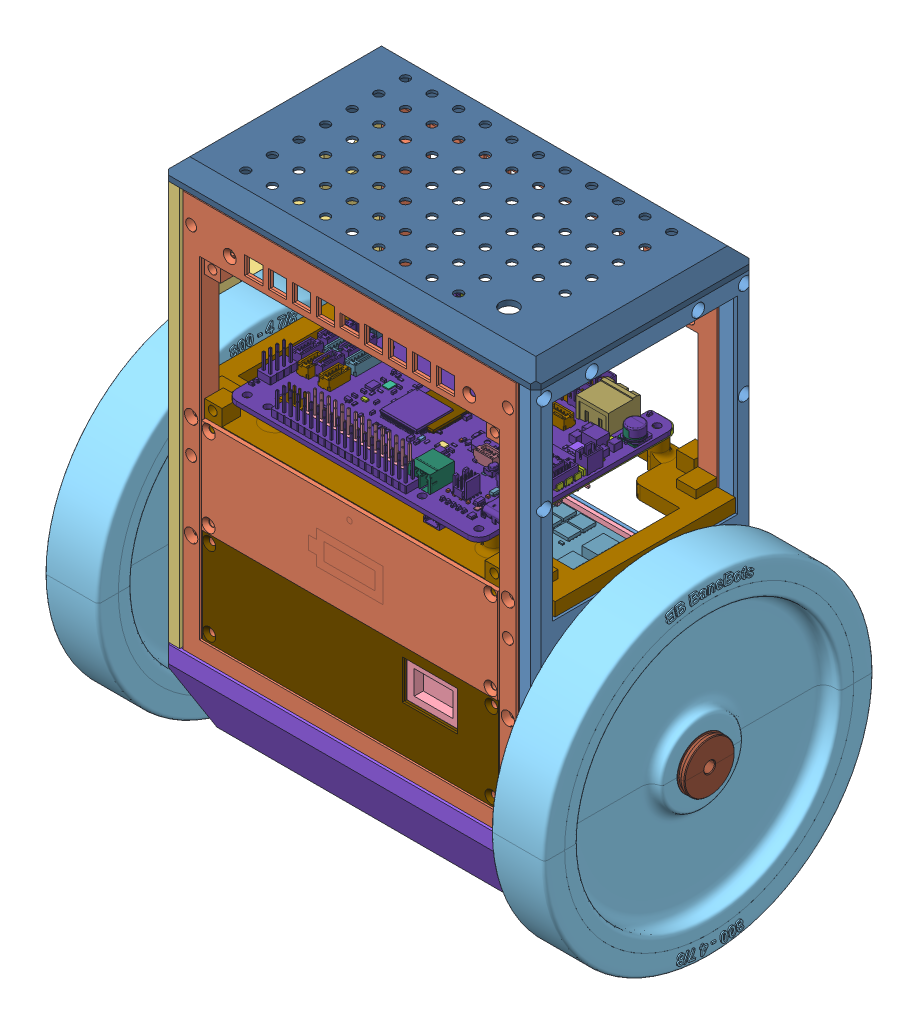
SolidWorks assembly twipr_v2, configuration Default. Lengths in mm. (continued)
Components (placement in the parent): (continued)
- robot-hub-1: robot-hub [Default] at (-323.8774 212.8203 108.5) x (-1 0 0) z (0 1 0) size (91.46 70 13.31) (continued)
  - robot-hub.step-1: robot-hub.step [Default] at origin size (91.46 70 13.31) (continued)
    - sk6812_side.step-1: sk6812_side.step [Default] at (75.35 -89.1 -1.05) x (0 -1 0) z (-1 0 0) size (4 2 1.6)
      - SOLID-45.step-1: SOLID-45.step [Default] at origin size (4 2 1.6)
    - R_0603_1608Metric.step-40: R_0603_1608Metric.step [Default] at (96 -111.5 -0.05) x (1 0 0) z (0 0 -1) size (1.6 0.8 0.45)
      - SOLID.step-1: SOLID.step [Default] at origin size (1.6 0.8 0.45)
    - R_0603_1608Metric.step-41: R_0603_1608Metric.step [Default] at (77.2 -90.65 -0.05) x (0 1 0) z (0 0 -1) size (1.6 0.8 0.45)
      - SOLID.step-1: SOLID.step [Default] at origin size (1.6 0.8 0.45)
    - C_0603_1608Metric.step-27: C_0603_1608Metric.step [Default] at (105.3 -137.6 -0.05) x (0 1 0) z (0 0 -1) size (1.6 0.8 0.8)
      - SOLID-1.step-1: SOLID-1.step [Default] at origin size (1.6 0.8 0.8)
    - STM32G031G6U6.step-2: STM32G031G6U6.step [Default] at (108.7 -137.5 -0.05) x (1 0 0) z (0 0 -1) size (4.1 4.1 0.6)
      - COMPOUND-31.step-1: COMPOUND-31.step [Default] at origin size (4.1 4.1 0.6)
    - SN74LVC3G17DCTR.step-1: SN74LVC3G17DCTR.step [Default] at (134.75 -142.2 -0.05) x (0 1 0) z (0 0 -1) size (4 2.95 1.3)
      - COMPOUND-46.step-1: COMPOUND-46.step [Default] at origin size (4 2.95 1.3)
    - R_0603_1608Metric.step-42: R_0603_1608Metric.step [Default] at (108.9 -109.7 -0.05) x (-1 0 0) z (0 0 -1) size (1.6 0.8 0.45)
      - SOLID.step-1: SOLID.step [Default] at origin size (1.6 0.8 0.45)
    - C_0805_2012Metric.step-8: C_0805_2012Metric.step [Default] at (94.8 -100.9 -0.05) x (0 1 0) z (0 0 -1) size (2 1.25 1.25)
      - SOLID-11.step-1: SOLID-11.step [Default] at origin size (2 1.25 1.25)
    - M24512-DFDW6TP.step-2: M24512-DFDW6TP.step [Default] at (121.95 -141.55 -0.05) x (1 0 0) z (0 0 -1) size (6.4 3 1.2)
      - COMPOUND-38.step-1: COMPOUND-38.step [Default] at origin size (6.4 3 1.2)
    - C_0603_1608Metric.step-28: C_0603_1608Metric.step [Default] at (101.6 -87.75 -0.05) x (1 0 0) z (0 0 -1) size (1.6 0.8 0.8)
      - SOLID-1.step-1: SOLID-1.step [Default] at origin size (1.6 0.8 0.8)
    - C_0603_1608Metric.step-29: C_0603_1608Metric.step [Default] at (108 -133.3 -0.05) x (0 -1 0) z (0 0 -1) size (1.6 0.8 0.8)
      - SOLID-1.step-1: SOLID-1.step [Default] at origin size (1.6 0.8 0.8)
    - R_0603_1608Metric.step-43: R_0603_1608Metric.step [Default] at (126.9 -130.4 -0.05) x (0 -1 0) z (0 0 -1) size (1.6 0.8 0.45)
      - SOLID.step-1: SOLID.step [Default] at origin size (1.6 0.8 0.45)
    - R_0603_1608Metric.step-44: R_0603_1608Metric.step [Default] at (141.135 -134.9385 -0.05) x (0 1 0) z (0 0 -1) size (1.6 0.8 0.45)
      - SOLID.step-1: SOLID.step [Default] at origin size (1.6 0.8 0.45)
    - SOT-23-6.step-3: SOT-23-6.step [Default] at (153.1 -91.8 -0.05) x (1 0 0) z (0 0 -1) size (2.8 2.9 1.55)
      - SOLID-24.step-1: SOLID-24.step [Default] at origin size (2.8 2.9 1.55)
    - R_0603_1608Metric.step-45: R_0603_1608Metric.step [Default] at (119.59 -119.2 -0.05) x (-1 0 0) z (0 0 -1) size (1.6 0.8 0.45)
      - SOLID.step-1: SOLID.step [Default] at origin size (1.6 0.8 0.45)
    - R_0603_1608Metric.step-46: R_0603_1608Metric.step [Default] at (128.5 -130.4 -0.05) x (0 -1 0) z (0 0 -1) size (1.6 0.8 0.45)
      - SOLID.step-1: SOLID.step [Default] at origin size (1.6 0.8 0.45)
    - R_0603_1608Metric.step-47: R_0603_1608Metric.step [Default] at (128.8 -109 -0.05) x (0 1 0) z (0 0 -1) size (1.6 0.8 0.45)
      - SOLID.step-1: SOLID.step [Default] at origin size (1.6 0.8 0.45)
    - C_0805_2012Metric.step-9: C_0805_2012Metric.step [Default] at (96.9 -100.9 -0.05) x (0 1 0) z (0 0 -1) size (2 1.25 1.25)
      - SOLID-11.step-1: SOLID-11.step [Default] at origin size (2 1.25 1.25)
    - R_0603_1608Metric.step-48: R_0603_1608Metric.step [Default] at (141.135 -138.0385 -0.05) x (0 -1 0) z (0 0 -1) size (1.6 0.8 0.45)
      - SOLID.step-1: SOLID.step [Default] at origin size (1.6 0.8 0.45)
    - SM04B-SRSS-TB_dark.step-3: SM04B-SRSS-TB_dark.step [Default] at (101.5 -142.1 0.2) x (-1 0 0) z (0 -1 0) size (6 2.96 4.95)
      - SOLID-37.step-1: SOLID-37.step [Default] at origin size (6 2.96 4.95)
    - C_0603_1608Metric.step-30: C_0603_1608Metric.step [Default] at (139.0125 -133.3 -0.05) x (0 1 0) z (0 0 -1) size (1.6 0.8 0.8)
      - SOLID-1.step-1: SOLID-1.step [Default] at origin size (1.6 0.8 0.8)
    - R_0603_1608Metric.step-49: R_0603_1608Metric.step [Default] at (152.7 -142.2 -0.05) x (1 0 0) z (0 0 -1) size (1.6 0.8 0.45)
      - SOLID.step-1: SOLID.step [Default] at origin size (1.6 0.8 0.45)
    - C_0805_2012Metric.step-10: C_0805_2012Metric.step [Default] at (85.75 -93.75 -0.05) x (1 0 0) z (0 0 -1) size (2 1.25 1.25)
      - SOLID-11.step-1: SOLID-11.step [Default] at origin size (2 1.25 1.25)
    - R_0603_1608Metric.step-50: R_0603_1608Metric.step [Default] at (127.7 -96.9 -0.05) x (1 0 0) z (0 0 -1) size (1.6 0.8 0.45)
      - SOLID.step-1: SOLID.step [Default] at origin size (1.6 0.8 0.45)
    - C_0805_2012Metric.step-11: C_0805_2012Metric.step [Default] at (100.75 -132.4 -0.05) x (1 0 0) z (0 0 -1) size (2 1.25 1.25)
      - SOLID-11.step-1: SOLID-11.step [Default] at origin size (2 1.25 1.25)
    - NCV8187AMLE330TCG.step-1: NCV8187AMLE330TCG.step [Default] at (96.2 -119.9 -0.05) x (-1 0 0) z (0 0 -1) size (3.1 3 1)
      - COMPOUND-47.step-1: COMPOUND-47.step [Default] at origin size (3.1 3 1)
    - R_0402_1005Metric.step-11: R_0402_1005Metric.step [Default] at (91.95 -87.35 -0.05) x (-1 0 0) z (0 0 -1) size (1 0.5 0.35)
      - SOLID-3.step-1: SOLID-3.step [Default] at origin size (1 0.5 0.35)
    - SOIC-16_3.9x9.9mm_P1.27mm.step-1: SOIC-16_3.9x9.9mm_P1.27mm.step [Default] at (96.9 -106.7 -0.05) x (0 1 0) z (0 0 -1) size (6 9.9 1.75)
      - SOLID-48.step-1: SOLID-48.step [Default] at origin size (6 9.9 1.75)
    - C_0603_1608Metric.step-31: C_0603_1608Metric.step [Default] at (96.8 -92.75 -0.05) x (-1 0 0) z (0 0 -1) size (1.6 0.8 0.8)
      - SOLID-1.step-1: SOLID-1.step [Default] at origin size (1.6 0.8 0.8)
    - R_0603_1608Metric.step-51: R_0603_1608Metric.step [Default] at (107.7 -107.2 -0.05) x (0 1 0) z (0 0 -1) size (1.6 0.8 0.45)
      - SOLID.step-1: SOLID.step [Default] at origin size (1.6 0.8 0.45)
    - R_0603_1608Metric.step-52: R_0603_1608Metric.step [Default] at (141.5 -130.7 -0.05) x (0 -1 0) z (0 0 -1) size (1.6 0.8 0.45)
      - SOLID.step-1: SOLID.step [Default] at origin size (1.6 0.8 0.45)
    - ECS-120-20-33-CKM-TR.step-1: ECS-120-20-33-CKM-TR.step [Default] at (104.7 -102.5 -0.05) x (0 1 0) z (0 0 -1) size (3.38 2.68 0.9)
      - COMPOUND-49.step-1: COMPOUND-49.step [Default] at origin size (3.38 2.68 0.9)
    - R_0603_1608Metric.step-53: R_0603_1608Metric.step [Default] at (93.5 -139.3 -0.05) x (0 -1 0) z (0 0 -1) size (1.6 0.8 0.45)
      - SOLID.step-1: SOLID.step [Default] at origin size (1.6 0.8 0.45)
    - C_0603_1608Metric.step-32: C_0603_1608Metric.step [Default] at (125.4 -99.5 -0.05) x (0 1 0) z (0 0 -1) size (1.6 0.8 0.8)
      - SOLID-1.step-1: SOLID-1.step [Default] at origin size (1.6 0.8 0.8)
    - R_0402_1005Metric.step-12: R_0402_1005Metric.step [Default] at (91.95 -88.35 -0.05) x (1 0 0) z (0 0 -1) size (1 0.5 0.35)
      - SOLID-3.step-1: SOLID-3.step [Default] at origin size (1 0.5 0.35)
    - 5033981892.step-1: 5033981892.step [Default] at (97.05 29.65 -154.55) x (0 -1 0) z (0 0 1) size (13.1 14.05 1.28)
      - COMPOUND-50.step-1: COMPOUND-50.step [Default] at origin size (13.1 14.05 1.28)
    - R_0603_1608Metric.step-54: R_0603_1608Metric.step [Default] at (131.9625 -136.35 -0.05) x (0 -1 0) z (0 0 -1) size (1.6 0.8 0.45)
      - SOLID.step-1: SOLID.step [Default] at origin size (1.6 0.8 0.45)
    - SOT-563.step-2: SOT-563.step [Default] at (89.5 -84.65 -0.05) x (-1 0 0) z (0 0 -1) size (1.6 1.6 0.63)
      - SOLID-29.step-1: SOLID-29.step [Default] at origin size (1.6 1.6 0.63)
    - R_0603_1608Metric.step-55: R_0603_1608Metric.step [Default] at (94.45 -93.2 -0.05) x (0 -1 0) z (0 0 -1) size (1.6 0.8 0.45)
      - SOLID.step-1: SOLID.step [Default] at origin size (1.6 0.8 0.45)
    - R_0603_1608Metric.step-56: R_0603_1608Metric.step [Default] at (123.9 -130.4 -0.05) x (0 -1 0) z (0 0 -1) size (1.6 0.8 0.45)
      - SOLID.step-1: SOLID.step [Default] at origin size (1.6 0.8 0.45)
    - R_0603_1608Metric.step-57: R_0603_1608Metric.step [Default] at (117 -100 -0.05) x (0 -1 0) z (0 0 -1) size (1.6 0.8 0.45)
      - SOLID.step-1: SOLID.step [Default] at origin size (1.6 0.8 0.45)
    - R_0603_1608Metric.step-58: R_0603_1608Metric.step [Default] at (91.7 -139.3 -0.05) x (0 -1 0) z (0 0 -1) size (1.6 0.8 0.45)
      - SOLID.step-1: SOLID.step [Default] at origin size (1.6 0.8 0.45)
    - R_0402_1005Metric.step-13: R_0402_1005Metric.step [Default] at (91.95 -89.35 -0.05) x (1 0 0) z (0 0 -1) size (1 0.5 0.35)
      - SOLID-3.step-1: SOLID-3.step [Default] at origin size (1 0.5 0.35)
    - sk6812_side.step-2: sk6812_side.step [Default] at (75.35 -96.1 -1.05) x (0 -1 0) z (-1 0 0) size (4 2 1.6)
      - SOLID-45.step-1: SOLID-45.step [Default] at origin size (4 2 1.6)
    - R_0603_1608Metric.step-59: R_0603_1608Metric.step [Default] at (118.6 -100 -0.05) x (0 -1 0) z (0 0 -1) size (1.6 0.8 0.45)
      - SOLID.step-1: SOLID.step [Default] at origin size (1.6 0.8 0.45)
    - C_0805_2012Metric.step-12: C_0805_2012Metric.step [Default] at (92.9 -119.9 -0.05) x (0 -1 0) z (0 0 -1) size (2 1.25 1.25)
      - SOLID-11.step-1: SOLID-11.step [Default] at origin size (2 1.25 1.25)
    - C_0805_2012Metric.step-13: C_0805_2012Metric.step [Default] at (103.5 -135.8 -0.05) x (0 1 0) z (0 0 -1) size (2 1.25 1.25)
      - SOLID-11.step-1: SOLID-11.step [Default] at origin size (2 1.25 1.25)
    - SM04B-SRSS-TB_dark.step-4: SM04B-SRSS-TB_dark.step [Default] at (159.3 -127.9 0.2) x (0 -1 0) z (1 0 0) size (6 2.96 4.95)
      - SOLID-37.step-1: SOLID-37.step [Default] at origin size (6 2.96 4.95)
    - C_0603_1608Metric.step-33: C_0603_1608Metric.step [Default] at (78.75 -90.65 -0.05) x (0 1 0) z (0 0 -1) size (1.6 0.8 0.8)
      - SOLID-1.step-1: SOLID-1.step [Default] at origin size (1.6 0.8 0.8)
    - SN74LVC3G17DCTR.step-2: SN74LVC3G17DCTR.step [Default] at (134.7125 -134.9 -0.05) x (0 1 0) z (0 0 -1) size (4 2.95 1.3)
      - COMPOUND-46.step-1: COMPOUND-46.step [Default] at origin size (4 2.95 1.3)
    - DMS0008A.step-1: DMS0008A.step [Default] at (85.1 -135.6 -0.05) x (-1 0 0) z (0 0 -1) size (3.3 3.3 0.8)
      - COMPOUND-51.step-1: COMPOUND-51.step [Default] at origin size (3.3 3.3 0.8)
    - TPS22975NDSGT.step-1: TPS22975NDSGT.step [Default] at (104.8 -88.5 -0.05) x (0 1 0) z (0 0 -1) size (2 2 0.78)
      - COMPOUND-52.step-1: COMPOUND-52.step [Default] at origin size (2 2 0.78)
    - R_0603_1608Metric.step-60: R_0603_1608Metric.step [Default] at (143.1 -130.7 -0.05) x (0 -1 0) z (0 0 -1) size (1.6 0.8 0.45)
      - SOLID.step-1: SOLID.step [Default] at origin size (1.6 0.8 0.45)
    - Fuse_1206_3216Metric.step-2: Fuse_1206_3216Metric.step [Default] at (107.4 -86.4 -0.05) x (0 1 0) z (0 0 -1) size (3.2 1.6 0.55)
      - SOLID-32.step-1: SOLID-32.step [Default] at origin size (3.2 1.6 0.55)
    - SM04B-SRSS-TB_dark.step-5: SM04B-SRSS-TB_dark.step [Default] at (94 -81 0.2) x (1 0 0) z (0 1 0) size (6 2.96 4.95)
      - SOLID-37.step-1: SOLID-37.step [Default] at origin size (6 2.96 4.95)
    - R_0603_1608Metric.step-61: R_0603_1608Metric.step [Default] at (115.7 -89.4 -0.05) x (-1 0 0) z (0 0 -1) size (1.6 0.8 0.45)
      - SOLID.step-1: SOLID.step [Default] at origin size (1.6 0.8 0.45)
    - R_0603_1608Metric.step-62: R_0603_1608Metric.step [Default] at (101.2 -129.6 -0.05) x (0 -1 0) z (0 0 -1) size (1.6 0.8 0.45)
      - SOLID.step-1: SOLID.step [Default] at origin size (1.6 0.8 0.45)
    - R_0603_1608Metric.step-63: R_0603_1608Metric.step [Default] at (148.335 -138.0385 -0.05) x (0 1 0) z (0 0 -1) size (1.6 0.8 0.45)
      - SOLID.step-1: SOLID.step [Default] at origin size (1.6 0.8 0.45)
    - PCT2075TP,147.step-2: PCT2075TP,147.step [Default] at (125 -105.6 -0.05) x (1 0 0) z (0 0 -1) size (3.1 2 0.8)
      - COMPOUND-44.step-1: COMPOUND-44.step [Default] at origin size (3.1 2 0.8)
    - R_0603_1608Metric.step-64: R_0603_1608Metric.step [Default] at (101.6 -89.35 -0.05) x (1 0 0) z (0 0 -1) size (1.6 0.8 0.45)
      - SOLID.step-1: SOLID.step [Default] at origin size (1.6 0.8 0.45)
    - R_0603_1608Metric.step-65: R_0603_1608Metric.step [Default] at (149.6 -109.1 -0.05) x (0 -1 0) z (0 0 -1) size (1.6 0.8 0.45)
      - SOLID.step-1: SOLID.step [Default] at origin size (1.6 0.8 0.45)
    - R_0603_1608Metric.step-66: R_0603_1608Metric.step [Default] at (153 -84.3 -0.05) x (0 1 0) z (0 0 -1) size (1.6 0.8 0.45)
      - SOLID.step-1: SOLID.step [Default] at origin size (1.6 0.8 0.45)
    - C_0603_1608Metric.step-34: C_0603_1608Metric.step [Default] at (132 -140.4 -0.05) x (0 1 0) z (0 0 -1) size (1.6 0.8 0.8)
      - SOLID-1.step-1: SOLID-1.step [Default] at origin size (1.6 0.8 0.8)
    - C_0603_1608Metric.step-35: C_0603_1608Metric.step [Default] at (151.45 -132.75 -0.05) x (-1 0 0) z (0 0 -1) size (1.6 0.8 0.8)
      - SOLID-1.step-1: SOLID-1.step [Default] at origin size (1.6 0.8 0.8)
    - R_0603_1608Metric.step-67: R_0603_1608Metric.step [Default] at (101.4 -101.2 -0.05) x (0 1 0) z (0 0 -1) size (1.6 0.8 0.45)
      - SOLID.step-1: SOLID.step [Default] at origin size (1.6 0.8 0.45)
    - R_0603_1608Metric.step-68: R_0603_1608Metric.step [Default] at (108.9 -111.2 -0.05) x (-1 0 0) z (0 0 -1) size (1.6 0.8 0.45)
      - SOLID.step-1: SOLID.step [Default] at origin size (1.6 0.8 0.45)
    - Fuse_1206_3216Metric.step-3: Fuse_1206_3216Metric.step [Default] at (90.5 -120.5 -0.05) x (0 -1 0) z (0 0 -1) size (3.2 1.6 0.55)
      - SOLID-32.step-1: SOLID-32.step [Default] at origin size (3.2 1.6 0.55)
    - robot-hub_rev3 PCB.step-1: robot-hub_rev3 PCB.step [Default] at origin size (90 70 1.66)
- bat_compartment-1: bat_compartment [Default] at (-442.6774 127.2203 0) x (1 0 0) z (0 0 -1) size (140 30 82)
- platform_control_v3_PanelMount-1: platform_control_v3_PanelMount [Default] at (-442.6774 200.8203 -0.1) size (140 12 82)
- marker_top-1: marker_top [Default] at (-442.6774 277.2203 0) size (140 14 82)
- T81H-RM41.stp-1: T81H-RM41.stp [Default] at (-368.6774 147.2203 0) x (0 0 -1) z (1 0 0) size (20.32 20.32 20.32)
- T81H-RM41.stp-2: T81H-RM41.stp [Default] at (-516.6774 147.2203 0) x (0 0 1) z (-1 0 0) size (20.32 20.32 20.32)
- bat_compartment_lid-1: bat_compartment_lid [Default] at (-442.6774 127.2203 0) x (1 0 0) z (0 0 -1) size (125.4 4 61.8)
- SE020A_01a-1: SE020A_01a [Default] at (-382.6774 147.2203 0) x (0 1 0) z (0 0 1) size (35.71 70 44.21)
- SE020A_01a-2: SE020A_01a [Default] at (-502.6774 147.2203 0) x (0 -1 0) z (0 0 1) size (35.71 70 44.21)
- bms-1: bms [Default] at (-259.9274 173.7203 54.5) x (-1 0 0) z (0 1 0) size (80 66.03 12.3)
- RS485-Splitter-2: RS485-Splitter [Default] at (-504.6774 320.2203 -75.5) x (0 -1 0) z (1 0 0) size (18 13.5 5.9)
- BMS_holder_big-1: BMS_holder_big [Default] at (-439.9274 169.7203 2) size (78 4 63)
- robot-hub_v4-1: robot-hub_v4 [Default] at (-293.0544 213.3846 93.2517) x (-1 0 0) z (0 1 0) size (95.3 75 13.31) (hidden)
- cover_1-3: cover_1 [Default] at (-442.6774 151.9703 40.7) x (-1 0 0) z (0 0 -1) size (111.2 35.5 3.2)
- cover_2-3: cover_2 [Default] at (-442.6774 151.9703 -40.7) size (111.2 35.5 3.2)
- Part1^twipr_v2-1: Part1^twipr_v2 [Default] at (-442.6774 200.8203 39.5) size (111.3 35.6 1.68) (virtual)
Mates (geometry in assembly coordinates):
- Parallel1: parallel anti-aligned: plane of brace_right-2 through (-379.6774 202.2203 0) normal (-1 0 0)
- Coincident4: coincident anti-aligned: plane of brace_right-2 through (-379.6774 202.2203 0) normal (0 0 -1)
- Coincident5: coincident aligned: plane of brace_right-2 through (-372.6774 127.2203 -41) normal (0 0 -1); plane of brace_front_led-1 through (-442.6774 202.2203 -41) normal (0 0 -1)
- Coincident6: coincident aligned: plane of brace_right-2 through (-372.6774 277.2203 41) normal (0 1 0); plane of brace_front_led-1 through (-505.6774 277.2203 -34) normal (0 1 0)
- Coincident7: coincident anti-aligned: plane of brace_right-2 through (-379.6774 202.2203 0) normal (-1 0 0); plane of brace_front_led-1 through (-379.6774 127.2203 -34) normal (1 0 0)
- Coincident8: coincident anti-aligned: plane of brace_front_led-1 through (-505.6774 127.2203 -34) normal (-1 0 0); plane of brace_left_display-2 through (-505.6774 202.2203 0) normal (1 0 0)
- Coincident9: coincident aligned: plane of brace_front_led-1 through (-505.6774 277.2203 -34) normal (0 1 0); plane of brace_left_display-2 through (-512.6774 277.2203 -41) normal (0 1 0)
- Coincident10: coincident aligned: plane of brace_front_led-1 through (-442.6774 202.2203 -41) normal (0 0 -1); plane of brace_left_display-2 through (-512.6774 127.2203 -41) normal (0 0 -1)
- Coincident12: coincident aligned: plane of brace_right-2 through (-372.6774 277.2203 41) normal (0 1 0); plane of brace_front_led-2 through (-379.6774 277.2203 34) normal (0 1 0)
- Parallel5: parallel anti-aligned: plane of brace_right-2 through (-372.6774 202.2203 0) normal (1 0 0); plane of banebots_4_78-1 through (-361.252 137.0603 10.16) normal (-1 0 0)
- Coincident25: coincident anti-aligned: plane of banebots_4_78-1 through (-368.872 147.2203 0) normal (0 0 -1)
- Coincident26: coincident aligned: plane of banebots_4_78-1 through (-368.872 147.2203 0) normal (0 1 0); plane of banebots_4_78-2 through (-516.2261 147.2203 0) normal (0 1 0)
- Coincident27: coincident anti-aligned: plane of banebots_4_78-1 through (-368.872 147.2203 0) normal (0 0 -1); plane of banebots_4_78-2 through (-516.2261 147.2203 0) normal (0 0 1)
- Coincident31: coincident anti-aligned: plane of brace_front_led-2 through (-379.6774 127.2203 34) normal (0 -1 0); plane of bat_compartment-1 through (-442.6774 127.2203 0) normal (0 1 0)
- Coincident36: coincident aligned: plane of brace_left_display-2 through (-512.6774 202.2203 0) normal (-1 0 0); plane of platform_control_v3_PanelMount-1 through (-512.6774 205.8203 33.8) normal (-1 0 0)
- Coincident38: coincident anti-aligned: plane of brace_right-2 through (-372.6774 277.2203 41) normal (0 1 0); plane of marker_top-1 through (-442.6774 277.2203 0) normal (0 -1 0)
- Coincident39: coincident aligned: plane of brace_front_led-1 through (-442.6774 202.2203 -41) normal (0 0 -1); plane of marker_top-1 through (-512.6774 279.2203 -41) normal (0 0 -1)
- Coincident40: coincident aligned: plane of brace_left_display-2 through (-512.6774 202.2203 0) normal (-1 0 0); plane of marker_top-1 through (-512.6774 279.2203 41) normal (-1 0 0)
- Coincident42: coincident anti-aligned: plane of robot-hub-1/robot-hub.step-1/robot-hub_rev3 PCB.step-1 through (-441.9229 212.8203 -3.7319) normal (0 -1 0); plane of platform_control_v3_PanelMount-1 through (-483.6774 212.8203 27.9) normal (0 1 0)
- Concentric7: concentric aligned: circle of robot-hub-1/robot-hub.step-1/robot-hub_rev3 PCB.step-1; circle of platform_control-1
- Concentric8: concentric aligned: circle of robot-hub-1/robot-hub.step-1/robot-hub_rev3 PCB.step-1; circle of platform_control-1
- Concentric11: concentric aligned: circle of brace_front-1; circle of platform_control-1
- Concentric274: concentric aligned: circle of brace_front-1; circle of platform_middle-1
- Coincident583: coincident aligned: plane of brace_right-2 through (-379.6774 202.2203 0) normal (0 0 -1); plane of T81H-RM41.stp-1 through (-368.6774 147.2203 0) normal (0 0 -1)
- Distance2: distance = 4 mm: point of T81H-RM41.stp-1; plane of brace_right-2 through (-372.6774 202.2203 0) normal (1 0 0)
- Coincident586: coincident aligned: plane of brace_left_display-2 through (-505.6774 202.2203 0) normal (0 0 1); plane of T81H-RM41.stp-2 through (-516.6774 147.2203 0) normal (0 0 1)
- Distance3: distance = 4 mm: point of T81H-RM41.stp-2; plane of brace_left_display-2 through (-512.6774 202.2203 0) normal (-1 0 0)
- Lock1: lock: unknown of banebots_4_78-1; unknown of T81H-RM41.stp-1
- Lock2: lock: unknown of banebots_4_78-2; unknown of T81H-RM41.stp-2
- Coincident592: coincident anti-aligned: plane of brace_front_led-1 through (-442.6774 202.2203 -34) normal (0 0 1); plane of platform_control_v3_PanelMount-1 through (-512.6774 205.8203 -34) normal (0 0 -1)
- Coincident593: coincident anti-aligned: plane of bat_compartment-1 through (-442.6774 123.2203 0) normal (0 1 0); plane of bat_compartment_lid-1 through (-442.6774 123.2203 0) normal (0 -1 0)
- Concentric275: concentric aligned: circle of bat_compartment-1; circle of bat_compartment_lid-1
- Concentric276: concentric aligned: circle of bat_compartment-1; circle of bat_compartment_lid-1
- Parallel8: parallel anti-aligned: plane of brace_right-2 through (-379.6774 202.2203 0) normal (-1 0 0); plane of platform_middle_big_bms-1 through (-379.7274 169.7203 34) normal (1 0 0)
- Coincident598: coincident anti-aligned: plane of brace_right-2 through (-378.6774 202.2203 0) normal (-1 0 0); plane of SE020A_01a-1 through (-378.6774 147.2203 -1) normal (1 0 0)
- Concentric281: concentric aligned: circle of brace_left-1; circle of SE020A_01a-1
- Parallel9: parallel aligned: plane of platform_middle_big_bms-1 through (-462.7274 87.6703 -21.5) normal (0 0 -1); plane of SE020A_01a-1 through (-403.6774 147.2203 -21.5) normal (0 0 -1)
- Coincident600: coincident anti-aligned: plane of brace_left_display-2 through (-506.6774 202.2203 0) normal (1 0 0); plane of SE020A_01a-2 through (-506.6774 147.2203 -1) normal (-1 0 0)
- Concentric282: concentric aligned: circle of brace_right-1; circle of SE020A_01a-2
- Parallel10: parallel aligned: plane of platform_middle_big_bms-1 through (-462.7274 87.6703 -21.5) normal (0 0 -1); plane of SE020A_01a-2 through (-481.6774 147.2203 -21.5) normal (0 0 -1)
- Coincident601: coincident aligned: plane of brace_left_display-2 through (-512.6774 127.2203 41) normal (0 0 1); plane of brace_front_led-2 through (-442.6774 202.2203 41) normal (0 0 1)
- Coincident602: coincident anti-aligned: plane of brace_right-2 through (-379.6774 202.2203 0) normal (-1 0 0); plane of brace_front_led-2 through (-379.6774 127.2203 34) normal (1 0 0)
- Coincident603: coincident aligned: plane of brace_front_led-2 through (-442.6774 202.2203 41) normal (0 0 1); plane of bat_compartment-1 through (-512.6774 120.2203 41) normal (0 0 1)
- Coincident604: coincident aligned: plane of brace_left_display-2 through (-512.6774 202.2203 0) normal (-1 0 0); plane of bat_compartment-1 through (-512.6774 120.2203 -41) normal (-1 0 0)
- Coincident605: coincident anti-aligned: plane of brace_front_led-2 through (-442.6774 202.2203 34) normal (0 0 -1); plane of platform_middle_big_bms-1 through (-386.8274 169.7203 34) normal (0 0 1)
- Parallel11: parallel anti-aligned: plane of platform_middle_big_bms-1 through (-442.7274 169.7203 0) normal (0 1 0); plane of bms-1 through (-439.9274 173.7203 2) normal (0 -1 0)
- Parallel12: parallel anti-aligned: plane of brace_right-2 through (-379.6774 202.2203 0) normal (-1 0 0); plane of bms-1 through (-399.9274 173.7203 -26.5) normal (1 0 0)
- Concentric289: concentric anti-aligned: circle of platform_middle_big_bms-1; circle of bms-1
- Concentric290: concentric anti-aligned: circle of platform_middle_big_bms-1; circle of bms-1
- Coincident610: coincident anti-aligned: plane of brace_left_display-2 through (-504.6774 202.2203 0) normal (1 0 0); plane of RS485-Splitter-2 through (-504.6774 191.2203 0) normal (-1 0 0)
- Concentric293: concentric anti-aligned: circle of brace_left_display-2; circle of RS485-Splitter-2
- Concentric294: concentric anti-aligned: circle of brace_left_display-2; circle of RS485-Splitter-2
- Coincident611: coincident anti-aligned: plane of platform_middle_big_bms-1 through (-442.7274 169.7203 0) normal (0 1 0); plane of BMS_holder_big-1 through (-403.9274 169.7203 -26.5) normal (0 -1 0)
- Concentric297: concentric aligned: circle of platform_middle_big_bms-1; circle of BMS_holder_big-1
- Concentric298: concentric aligned: circle of platform_middle_big_bms-1; circle of BMS_holder_big-1
- Coincident613: coincident anti-aligned: plane of bms-1 through (-439.9274 173.7203 2) normal (0 -1 0); plane of BMS_holder_big-1 through (-403.9274 173.7203 -26.5) normal (0 1 0)
- Parallel13: parallel anti-aligned: plane of platform_control_v3_PanelMount-1 through (-442.6774 205.8203 -0.1) normal (0 1 0); plane of robot-hub_v4-1 through (-444.2861 213.3846 -0.6198) normal (0 -1 0)
- Parallel14: parallel aligned: plane of brace_right-2 through (-372.6774 202.2203 0) normal (1 0 0); plane of robot-hub_v4-1 through (-397.5494 213.3846 -33.4333) normal (1 0 0)
- Coincident614: coincident anti-aligned: plane of brace_front_led-2 through (-442.6774 202.2203 39.5) normal (0 0 1); plane of cover_1-3 through (-442.6774 151.9703 39.5) normal (0 0 -1)
- Concentric299: concentric anti-aligned: circle of brace_front_led-2; circle of cover_1-3
- Concentric300: concentric anti-aligned: circle of brace_front_led-2; circle of cover_1-3
- Coincident616: coincident anti-aligned: plane of brace_front_led-1 through (-442.6774 202.2203 -39.5) normal (0 0 -1); plane of cover_2-3 through (-442.6774 151.9703 -39.5) normal (0 0 1)
- Concentric301: concentric aligned: circle of brace_front_led-1; circle of cover_2-3
- Concentric302: concentric aligned: circle of brace_front_led-1; circle of cover_2-3
- InPlace1: in place: plane of platform_control_v3_PanelMount-1 through (-386.7774 200.8203 39.5) normal (0 0 1); plane of ? through (0 0 39.5) normal (0 0 1); moOrthogonalPlaneRef_w of platform_control_v3_PanelMount-1 through (-386.7774 200.8203 39.5) normal (0 0 1); plane of ? through (0 0 39.5) normal (0 1 0); plane of platform_control_v3_PanelMount-1 through (-386.7774 200.8203 39.5) normal (0 0 1); plane of ? through (0 0 39.5) normal (1 0 0); plane of platform_control_v3_PanelMount-1 through (-386.7774 200.8203 39.5) normal (0 0 1); unknown of Part1^twipr_v2-1
- Coincident617: coincident aligned: plane of platform_control_v3_PanelMount-1; plane of Part1^twipr_v2-1
- Coincident618: coincident aligned: moOrthogonalPlaneRef_w of platform_control_v3_PanelMount-1 through (-442.6774 200.8203 39.5) normal (0 1 0); plane of Part1^twipr_with_additions-1 through (-442.6774 200.8203 39.5) normal (0 1 0)
- Coincident619: coincident anti-aligned: moOrthogonalPlaneRef_w of platform_control_v3_PanelMount-1 through (-442.6774 200.8203 39.5) normal (-1 0 0); plane of Part1^twipr_with_additions-1 through (-442.6774 200.8203 39.5) normal (1 0 0)
